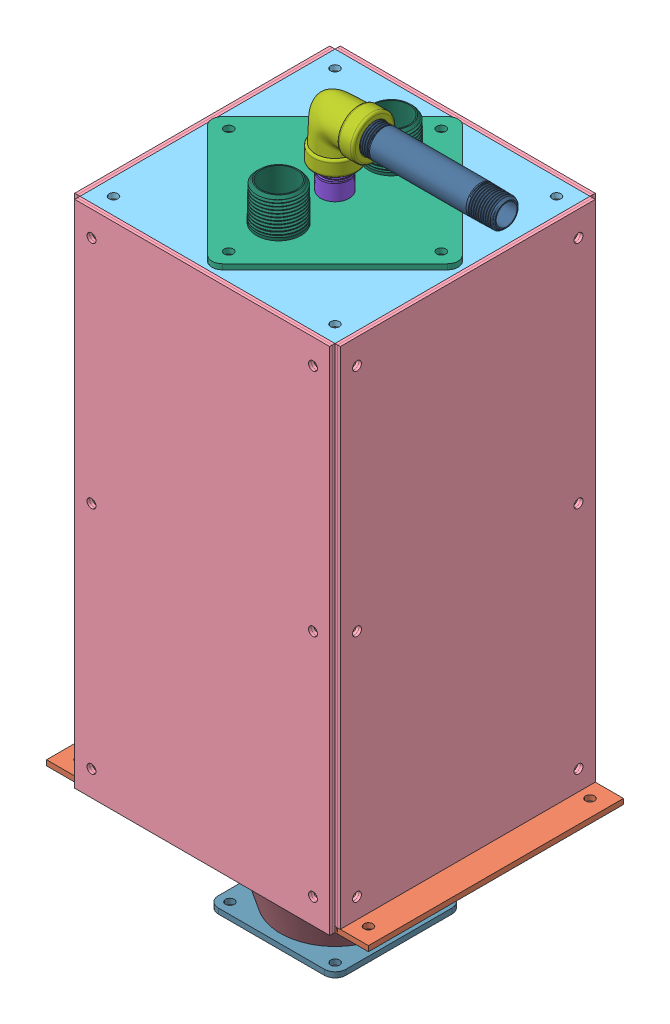
SolidWorks assembly dryer stand alone, configuration Default. Lengths in mm.
Overall size (209.74 423.31 158.7).
29 component instances, 15 part files, 74 mates.
Components (placement in the parent):
- tube-1: tube [Default] at (103.5422 61.3012 185.6839) size (164.34 304.8 101.6)
- flange rev01-1: flange rev01 [Default] at (103.5422 61.3012 185.6839) x (-1 0 0) z (0 0 -1) size (192.4 3.17 152.4)
- HFS5-2020-299-1: HFS5-2020-299 [Default] at (169.7422 63.9262 119.4839) x (-1 0 0) z (0 -1 0) size (20 20 298.45)
- HFS5-2020-299-2: HFS5-2020-299 [Default] at (37.3422 63.9262 119.4839) x (-1 0 0) z (0 -1 0) size (20 20 298.45)
- HFS5-2020-299-3: HFS5-2020-299 [Default] at (169.7422 63.9262 251.8839) x (-1 0 0) z (0 -1 0) size (20 20 298.45)
- HFS5-2020-299-4: HFS5-2020-299 [Default] at (37.3422 363.4762 251.8839) x (-1 0 0) z (0 1 0) size (20 20 298.45)
- side plate 1_16-1: side plate 1_16 [Default] at (103.5422 213.7012 263.4587) x (-1 0 0) z (0 0 -1) size (152.4 304.8 1.57)
- side plate 1_16-2: side plate 1_16 [Default] at (103.5422 213.7012 265.0335) x (-1 0 0) z (0 0 -1) size (152.4 304.8 1.57)
- flange rev02-1: flange rev02 [Default] at (103.5422 362.9262 185.6839) x (-1 0 0) z (0 0 -1) size (152.4 3.17 152.4)
- top cover-1: top cover [Default] at (103.5422 369.2762 185.6839) x (-0.707107 0 -0.707107) z (0 -1 0) size (107.76 107.76 3.17)
- 4452K413_TYPE 316 STAINLESS STL THREADED PIPE FITTING-2: 4452K413_TYPE 316 STAINLESS STL THREADED PIPE FITTING [4452K413] at (103.5422 407.8982 185.6839) x (-1 0 0) z (0 0 1) size (37.28 37.03 30.11)
- 4548K159_STD-WALL TYPE 316-316L SS THRD PIPE NIPPLE-1: 4548K159_STD-WALL TYPE 316-316L SS THRD PIPE NIPPLE [4548K159] at (103.5422 292.6762 185.6839) x (0 1 0) z (0 0 1) size (203.35 17.91 17.78)
- 4464K498_TYPE 304 STAINLESS STL THREADED PIPE FITTING-1: 4464K498_TYPE 304 STAINLESS STL THREADED PIPE FITTING [4464K498] at (103.5422 180.2482 185.6839) x (-0.837169 0 -0.546944) z (0 1 0) size (25.91 25.91 21.03)
- 4548K145_STD-WALL TYPE 316-316L SS THRD PIPE NIPPLE-2: 4548K145_STD-WALL TYPE 316-316L SS THRD PIPE NIPPLE [4548K145] at (161.6142 407.8982 185.6839) x (1 0 0) z (0 -0.851872 -0.523749) size (89.04 17.99 18.06)
- heater band-1: heater band [Default] at (103.5422 257.8762 185.6839) size (116.47 50.8 107.95)
- heater band-2: heater band [Default] at (103.5422 132.2762 185.6839) size (116.47 50.8 107.95)
- heater band-3: heater band [Default] at (103.5422 69.4762 185.6839) size (116.47 50.8 107.95)
- heater band-4: heater band [Default] at (103.5422 195.0762 185.6839) size (116.47 50.8 107.95)
- bottom cover-1: bottom cover [Default] at (103.6306 61.3012 185.6839) x (-0.707107 0 -0.707107) z (0 -1 0) size (107.76 107.76 3.17)
- nozzle reduction-1: nozzle reduction [Default] at (103.6306 61.3012 185.6839) x (-0.837169 0 -0.546944) z (-0.546944 0 0.837169) size (101.6 63.5 101.6)
- 2.5 in bracket-1: 2.5 in bracket [Default] at (103.6306 -2.1988 185.6839) size (76.2 3.17 76.2)
- side plate 1_16-7: side plate 1_16 [Default] at (103.5422 213.7012 107.9091) size (152.4 304.8 1.57)
- side plate 1_16-8: side plate 1_16 [Default] at (103.5422 213.7012 106.3343) size (152.4 304.8 1.57)
- 9157K150_STD-WALL 304-304L SS THRD ONE END PIPE NIPPLE-1: 9157K150_STD-WALL 304-304L SS THRD ONE END PIPE NIPPLE [9157K15] at (103.5422 378.8012 152.0289) x (0 1 0) z (-0.332767 0 0.943009) size (25.49 27.89 27.84)
- 9157K150_STD-WALL 304-304L SS THRD ONE END PIPE NIPPLE-2: 9157K150_STD-WALL 304-304L SS THRD ONE END PIPE NIPPLE [9157K15] at (103.5422 378.8012 219.3389) x (0 1 0) z (-0.546944 0 0.837169) size (25.49 27.89 27.84)
- side plate 1_16-9: side plate 1_16 [Default] at (182.8918 213.7012 185.6839) x (0 0 1) z (-1 0 0) size (152.4 304.8 1.57)
- side plate 1_16-10: side plate 1_16 [Default] at (181.317 213.7012 185.6839) x (0 0 1) z (-1 0 0) size (152.4 304.8 1.57)
- side plate 1_16-11: side plate 1_16 [Default] at (27.3422 213.7012 185.6839) x (0 0 1) z (-1 0 0) size (152.4 304.8 1.57)
- side plate 1_16-12: side plate 1_16 [Default] at (25.7674 213.7012 185.6839) x (0 0 1) z (-1 0 0) size (152.4 304.8 1.57)
Mates (geometry in assembly coordinates):
- Concentric1: concentric aligned: cylinder of tube-1 through (103.5422 366.1012 185.6839) axis (0 -1 0) radius 50.8; cylinder of flange rev01-1 through (103.5422 64.4762 185.6839) axis (0 -1 0) radius 50.8
- Coincident1: coincident anti-aligned: circle of tube-1; plane of flange rev01-1 through (103.5422 61.3012 185.6839) normal (0 -1 0)
- Coincident2: coincident anti-aligned: plane of flange rev01-1 through (103.5422 64.4762 185.6839) normal (0 1 0); plane of HFS5-2020-299-1 through (178.7422 64.4762 128.4839) normal (0 -1 0)
- Coincident3: coincident aligned: plane of flange rev01-1 through (179.7422 64.4762 109.4839) normal (0 0 -1); plane of HFS5-2020-299-1 through (160.7422 362.9262 109.4839) normal (0 0 -1)
- Coincident5: coincident anti-aligned: plane of flange rev01-1 through (103.5422 64.4762 185.6839) normal (0 1 0); plane of HFS5-2020-299-2 through (46.3422 64.4762 128.4839) normal (0 -1 0)
- Coincident6: coincident aligned: plane of flange rev01-1 through (179.7422 64.4762 109.4839) normal (0 0 -1); plane of HFS5-2020-299-2 through (28.3422 362.9262 109.4839) normal (0 0 -1)
- Coincident8: coincident anti-aligned: plane of flange rev01-1 through (103.5422 64.4762 185.6839) normal (0 1 0); plane of HFS5-2020-299-3 through (178.7422 64.4762 260.8839) normal (0 -1 0)
- Coincident10: coincident aligned: plane of flange rev01-1 through (179.7422 64.4762 261.8839) normal (0 0 1); plane of HFS5-2020-299-3 through (178.7422 362.9262 261.8839) normal (0 0 1)
- Coincident11: coincident anti-aligned: plane of flange rev01-1 through (103.5422 64.4762 185.6839) normal (0 1 0); plane of HFS5-2020-299-4 through (46.3422 64.4762 242.8839) normal (0 -1 0)
- Coincident12: coincident aligned: plane of flange rev01-1 through (179.7422 64.4762 261.8839) normal (0 0 1); plane of HFS5-2020-299-4 through (40.3422 64.4762 261.8839) normal (0 0 1)
- Coincident14: coincident anti-aligned: plane of side plate 1_16-1 through (103.5422 213.7012 263.4587) normal (0 0 1); plane of side plate 1_16-2 through (103.5422 213.7012 263.4587) normal (0 0 -1)
- Coincident15: coincident aligned: plane of side plate 1_16-1 through (179.7422 366.1012 261.8839) normal (0 1 0); plane of side plate 1_16-2 through (179.7422 366.1012 263.4587) normal (0 1 0)
- Coincident16: coincident aligned: plane of side plate 1_16-1 through (179.7422 61.3012 261.8839) normal (1 0 0); plane of side plate 1_16-2 through (179.7422 61.3012 263.4587) normal (1 0 0)
- Coincident17: coincident anti-aligned: plane of HFS5-2020-299-3 through (166.7422 362.9262 261.8839) normal (0 0 1); plane of side plate 1_16-1 through (103.5422 213.7012 261.8839) normal (0 0 -1)
- Coincident18: coincident aligned: plane of flange rev01-1 through (103.5422 61.3012 185.6839) normal (0 -1 0); plane of side plate 1_16-1 through (179.7422 61.3012 261.8839) normal (0 -1 0)
- Coincident19: coincident aligned: plane of HFS5-2020-299-3 through (179.7422 362.9262 254.8839) normal (1 0 0); plane of side plate 1_16-1 through (179.7422 61.3012 261.8839) normal (1 0 0)
- Coincident33: coincident aligned: plane of side plate 1_16-1 through (179.7422 366.1012 261.8839) normal (0 1 0); plane of flange rev02-1 through (103.5422 366.1012 185.6839) normal (0 1 0)
- Coincident34: coincident aligned: plane of HFS5-2020-299-3 through (179.7422 362.9262 254.8839) normal (1 0 0); plane of flange rev02-1 through (179.7422 366.1012 109.4839) normal (1 0 0)
- Coincident35: coincident anti-aligned: plane of side plate 1_16-1 through (103.5422 213.7012 261.8839) normal (0 0 -1); plane of flange rev02-1 through (179.7422 366.1012 261.8839) normal (0 0 1)
- Concentric9: concentric anti-aligned: cylinder of top cover-1 through (103.5422 369.2772 185.6839) axis (0 -1 0) radius 8.5725; cylinder of 4548K159_STD-WALL TYPE 316-316L SS THRD PIPE NIPPLE-1 through (103.5422 292.6762 185.6839) axis (0 1 0) radius 8.5725
- Distance4: distance = 25 mm aligned: plane of 4548K159_STD-WALL TYPE 316-316L SS THRD PIPE NIPPLE-1 through (103.5422 394.2762 185.6839) normal (0 1 0); plane of top cover-1 through (103.5422 369.2762 185.6839) normal (0 1 0)
- Concentric10: concentric aligned: cylinder of 4452K413_TYPE 316 STAINLESS STL THREADED PIPE FITTING-2 through (103.5422 384.2762 185.6839) axis (0 1 0) radius 12.954; cylinder of 4548K159_STD-WALL TYPE 316-316L SS THRD PIPE NIPPLE-1 through (103.5422 292.6762 185.6839) axis (0 1 0) radius 8.5725
- Distance5: distance = 15 mm anti-aligned: plane of 4452K413_TYPE 316 STAINLESS STL THREADED PIPE FITTING-2 through (103.5422 384.2762 185.6839) normal (0 -1 0); plane of top cover-1 through (103.5422 369.2762 185.6839) normal (0 1 0)
- Coincident38: coincident anti-aligned: plane of flange rev02-1 through (103.5422 366.1012 185.6839) normal (0 1 0); plane of top cover-1 through (103.5422 366.1012 185.6839) normal (0 -1 0)
- Concentric11: concentric aligned: cylinder of 4548K159_STD-WALL TYPE 316-316L SS THRD PIPE NIPPLE-1 through (103.5422 292.6762 185.6839) axis (0 1 0) radius 8.5725; cylinder of 4464K498_TYPE 304 STAINLESS STL THREADED PIPE FITTING-1 through (103.5422 195.7422 185.6839) axis (0 1 0) radius 12.954
- Distance6: distance = 10 mm anti-aligned: plane of 4548K159_STD-WALL TYPE 316-316L SS THRD PIPE NIPPLE-1 through (103.5422 191.0762 185.6839) normal (0 -1 0); plane of 4464K498_TYPE 304 STAINLESS STL THREADED PIPE FITTING-1 through (103.5422 201.0762 185.6839) normal (0 1 0)
- Concentric12: concentric anti-aligned: cylinder of 4452K413_TYPE 316 STAINLESS STL THREADED PIPE FITTING-2 through (127.1642 407.8982 185.6839) axis (-1 0 0) radius 12.954; cylinder of 4548K145_STD-WALL TYPE 316-316L SS THRD PIPE NIPPLE-2 through (161.6142 407.8982 185.6839) axis (1 0 0) radius 8.5725
- Distance7: distance = 10 mm anti-aligned: plane of 4548K145_STD-WALL TYPE 316-316L SS THRD PIPE NIPPLE-2 through (117.1642 407.8982 185.6839) normal (-1 0 0); plane of 4452K413_TYPE 316 STAINLESS STL THREADED PIPE FITTING-2 through (127.1642 407.8982 185.6839) normal (1 0 0)
- Concentric13: concentric aligned: cylinder of tube-1 through (103.5422 366.1012 185.6839) axis (0 -1 0) radius 50.8; cylinder of heater band-3 through (103.5422 120.2762 185.6839) axis (0 -1 0) radius 50.8
- Concentric14: concentric aligned: cylinder of tube-1 through (103.5422 366.1012 185.6839) axis (0 -1 0) radius 50.8; cylinder of heater band-2 through (103.5422 183.0762 185.6839) axis (0 -1 0) radius 50.8
- Concentric15: concentric aligned: cylinder of tube-1 through (103.5422 366.1012 185.6839) axis (0 -1 0) radius 50.8; cylinder of heater band-4 through (103.5422 245.8762 185.6839) axis (0 -1 0) radius 50.8
- Concentric16: concentric aligned: cylinder of tube-1 through (103.5422 366.1012 185.6839) axis (0 -1 0) radius 50.8; cylinder of heater band-1 through (103.5422 308.6762 185.6839) axis (0 -1 0) radius 50.8
- Distance8: distance = 5 mm anti-aligned: plane of heater band-3 through (103.5422 69.4762 185.6839) normal (0 -1 0); plane of flange rev01-1 through (103.5422 64.4762 185.6839) normal (0 1 0)
- Distance9: distance = 12 mm anti-aligned: plane of heater band-2 through (103.5422 132.2762 185.6839) normal (0 -1 0); plane of heater band-3 through (103.5422 120.2762 185.6839) normal (0 1 0)
- Distance10: distance = 12 mm anti-aligned: plane of heater band-2 through (103.5422 183.0762 185.6839) normal (0 1 0); plane of heater band-4 through (103.5422 195.0762 185.6839) normal (0 -1 0)
- Distance11: distance = 12 mm anti-aligned: plane of heater band-4 through (103.5422 245.8762 185.6839) normal (0 1 0); plane of heater band-1 through (103.5422 257.8762 185.6839) normal (0 -1 0)
- Coincident49: coincident aligned: plane of heater band-2 through (157.1424 183.0762 176.1589) normal (0 0 -1); plane of heater band-3 through (157.1424 120.2762 176.1589) normal (0 0 -1)
- Coincident50: coincident aligned: plane of heater band-2 through (157.1424 183.0762 176.1589) normal (0 0 -1); plane of heater band-4 through (157.1424 245.8762 176.1589) normal (0 0 -1)
- Coincident51: coincident aligned: plane of heater band-1 through (157.1424 308.6762 176.1589) normal (0 0 -1); plane of heater band-4 through (157.1424 245.8762 176.1589) normal (0 0 -1)
- Parallel5: parallel anti-aligned: plane of HFS5-2020-299-1 through (166.7422 362.9262 129.4839) normal (0 0 1); plane of heater band-3 through (157.1424 120.2762 176.1589) normal (0 0 -1)
- Coincident53: coincident anti-aligned: plane of flange rev01-1 through (103.5422 61.3012 185.6839) normal (0 -1 0); plane of bottom cover-1 through (103.6306 61.3012 185.6839) normal (0 1 0)
- Coincident54: coincident anti-aligned: plane of tube-1 through (103.5422 61.3012 185.6839) normal (0 -1 0); plane of nozzle reduction-1 through (103.6306 61.3012 185.6839) normal (0 1 0)
- Coincident55: coincident aligned: cylinder of bottom cover-1 through (103.6306 61.3022 185.6839) axis (0 -1 0) radius 50.8; circle of nozzle reduction-1
- Coincident56: coincident aligned: circle of nozzle reduction-1; cylinder of 2.5 in bracket-1 through (103.6306 0.9762 185.6839) axis (0 -1 0) radius 31.75
- Coincident57: coincident aligned: plane of nozzle reduction-1 through (103.6306 -2.1988 185.6839) normal (0 -1 0); plane of 2.5 in bracket-1 through (103.6306 -2.1988 185.6839) normal (0 -1 0)
- Parallel6: parallel: line of flange rev01-1 through (199.7422 61.3012 109.4839) axis (-1 0 0); plane of 2.5 in bracket-1 through (65.5306 0.9762 147.5839) normal (0 0 -1)
- Concentric20: concentric aligned: cylinder of tube-1 through (103.5422 366.1012 185.6839) axis (0 -1 0) radius 50.8; cylinder of top cover-1 through (103.5422 369.2772 185.6839) axis (0 -1 0) radius 8.5725
- Angle1: planar angle = 0.785398 rad aligned: plane of top cover-1 through (27.3422 366.1012 185.6839) normal (-0.707107 0 -0.707107); plane of flange rev02-1 through (27.3422 366.1012 109.4839) normal (-1 0 0)
- Coincident73: coincident anti-aligned: plane of side plate 1_16-7 through (103.5422 213.7012 107.9091) normal (0 0 -1); plane of side plate 1_16-8 through (103.5422 213.7012 107.9091) normal (0 0 1)
- Coincident74: coincident aligned: plane of side plate 1_16-7 through (27.3422 61.3012 109.4839) normal (-1 0 0); plane of side plate 1_16-8 through (27.3422 61.3012 107.9091) normal (-1 0 0)
- Coincident75: coincident aligned: plane of side plate 1_16-7 through (27.3422 366.1012 109.4839) normal (0 1 0); plane of side plate 1_16-8 through (27.3422 366.1012 107.9091) normal (0 1 0)
- Coincident76: coincident aligned: plane of flange rev02-1 through (103.5422 366.1012 185.6839) normal (0 1 0); plane of side plate 1_16-7 through (27.3422 366.1012 109.4839) normal (0 1 0)
- Coincident77: coincident anti-aligned: plane of HFS5-2020-299-1 through (160.7422 362.9262 109.4839) normal (0 0 -1); plane of side plate 1_16-7 through (103.5422 213.7012 109.4839) normal (0 0 1)
- Concentric21: concentric anti-aligned: cylinder of top cover-1 through (103.5422 369.2772 152.0289) axis (0 -1 0) radius 13.335; cylinder of 9157K150_STD-WALL 304-304L SS THRD ONE END PIPE NIPPLE-1 through (103.5422 366.1012 152.0289) axis (0 1 0) radius 13.335
- Coincident79: coincident aligned: circle of top cover-1; plane of 9157K150_STD-WALL 304-304L SS THRD ONE END PIPE NIPPLE-1 through (103.5422 366.1012 152.0289) normal (0 -1 0)
- Coincident80: coincident aligned: circle of top cover-1; plane of 9157K150_STD-WALL 304-304L SS THRD ONE END PIPE NIPPLE-2 through (103.5422 366.1012 219.3389) normal (0 -1 0)
- Concentric22: concentric anti-aligned: cylinder of top cover-1 through (103.5422 369.2772 219.3389) axis (0 -1 0) radius 13.335; cylinder of 9157K150_STD-WALL 304-304L SS THRD ONE END PIPE NIPPLE-2 through (103.5422 366.1012 219.3389) axis (0 1 0) radius 13.335
- Parallel10: parallel aligned: plane of side plate 1_16-2 through (103.5422 213.7012 265.0335) normal (0 0 1); plane of 4452K413_TYPE 316 STAINLESS STL THREADED PIPE FITTING-2 through (103.5422 407.8982 185.6839) normal (0 0 1)
- Parallel11: parallel aligned: plane of side plate 1_16-2 through (103.5422 213.7012 265.0335) normal (0 0 1); plane of assembly through (0 0 0) normal (0 0 1)
- Concentric23: concentric anti-aligned: cylinder of flange rev01-1 through (103.5422 61.3002 122.1839) axis (0 1 0) radius 2.665; cylinder of bottom cover-1 through (103.5422 61.3022 122.1839) axis (0 -1 0) radius 2.665
- Concentric24: concentric anti-aligned: cylinder of flange rev01-1 through (167.0422 61.3002 185.6839) axis (0 1 0) radius 2.665; cylinder of bottom cover-1 through (167.0422 61.3022 185.6839) axis (0 -1 0) radius 2.665
- Coincident81: coincident anti-aligned: plane of HFS5-2020-299-1 through (179.7422 362.9262 110.4839) normal (1 0 0); plane of side plate 1_16-10 through (179.7422 213.7012 185.6839) normal (-1 0 0)
- Parallel12: parallel anti-aligned: plane of side plate 1_16-1 through (103.5422 213.7012 261.8839) normal (0 0 -1); plane of side plate 1_16-10 through (179.7422 61.3012 261.8839) normal (0 0 1)
- Coincident83: coincident aligned: plane of flange rev02-1 through (103.5422 366.1012 185.6839) normal (0 1 0); plane of side plate 1_16-10 through (179.7422 366.1012 109.4839) normal (0 1 0)
- Coincident84: coincident anti-aligned: plane of side plate 1_16-1 through (103.5422 213.7012 261.8839) normal (0 0 -1); plane of side plate 1_16-10 through (179.7422 61.3012 261.8839) normal (0 0 1)
- Coincident85: coincident anti-aligned: plane of side plate 1_16-9 through (181.317 213.7012 185.6839) normal (-1 0 0); plane of side plate 1_16-10 through (181.317 213.7012 185.6839) normal (1 0 0)
- Concentric25: concentric aligned: cylinder of side plate 1_16-9 through (181.316 351.1012 119.4839) axis (1 0 0) radius 2.665; cylinder of side plate 1_16-10 through (179.7412 351.1012 119.4839) axis (1 0 0) radius 2.665
- Concentric26: concentric aligned: cylinder of side plate 1_16-9 through (181.316 351.1012 251.8839) axis (1 0 0) radius 2.665; cylinder of side plate 1_16-10 through (179.7412 351.1012 251.8839) axis (1 0 0) radius 2.665
- Coincident86: coincident anti-aligned: plane of HFS5-2020-299-4 through (27.3422 64.4762 242.8839) normal (-1 0 0); plane of side plate 1_16-11 through (27.3422 213.7012 185.6839) normal (1 0 0)
- Coincident87: coincident aligned: plane of flange rev02-1 through (103.5422 366.1012 185.6839) normal (0 1 0); plane of side plate 1_16-11 through (25.7674 366.1012 109.4839) normal (0 1 0)
- Coincident88: coincident anti-aligned: plane of side plate 1_16-7 through (103.5422 213.7012 109.4839) normal (0 0 1); plane of side plate 1_16-11 through (25.7674 61.3012 109.4839) normal (0 0 -1)
- Coincident89: coincident anti-aligned: plane of side plate 1_16-11 through (25.7674 213.7012 185.6839) normal (-1 0 0); plane of side plate 1_16-12 through (25.7674 213.7012 185.6839) normal (1 0 0)
- Concentric27: concentric aligned: cylinder of side plate 1_16-11 through (25.7664 351.1012 251.8839) axis (1 0 0) radius 2.665; cylinder of side plate 1_16-12 through (24.1916 351.1012 251.8839) axis (1 0 0) radius 2.665
- Concentric28: concentric aligned: cylinder of side plate 1_16-11 through (25.7664 351.1012 119.4839) axis (1 0 0) radius 2.665; cylinder of side plate 1_16-12 through (24.1916 351.1012 119.4839) axis (1 0 0) radius 2.665
